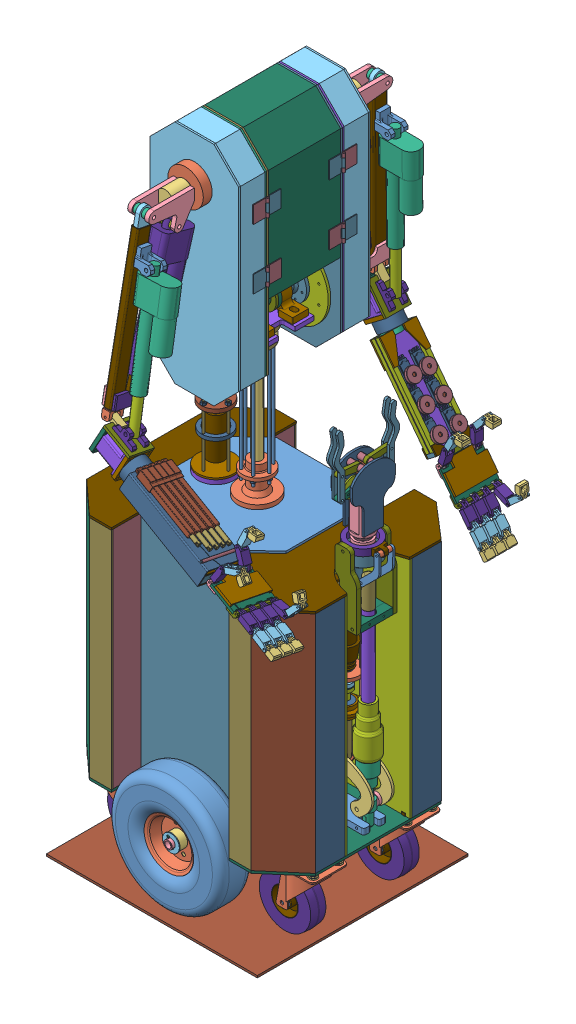
SolidWorks assembly sorbot, configuration По умолчанию. Lengths in mm. (continued)
Components (placement in the parent): (continued)
- bolt1-10: bolt1 [По умолчанию] at (-181.6432 28.2059 -219.1307) x (0.546944 0 -0.837169) z (-0.837169 0 -0.546944) size (14 40.5 16.17)
- bolt1-11: bolt1 [По умолчанию] at (-181.4767 28.2059 -278.9161) x (0.546944 0 -0.837169) z (-0.837169 0 -0.546944) size (14 40.5 16.17)
- bolt1-12: bolt1 [По умолчанию] at (-260.5141 28.2059 -278.9485) x (0.546944 0 -0.837169) z (-0.837169 0 -0.546944) size (14 40.5 16.17)
- bolt1-13: bolt1 [По умолчанию] at (-260.8842 28.1192 -54.1025) x (-0.546944 0 0.837169) z (0.837169 0 0.546944) size (14 40.5 16.17)
- bolt1-14: bolt1 [По умолчанию] at (-181.8952 28.1192 -54.0898) x (-0.546944 0 0.837169) z (0.837169 0 0.546944) size (14 40.5 16.17)
- bolt1-15: bolt1 [По умолчанию] at (-260.8825 28.1192 5.6198) x (-0.546944 0 0.837169) z (0.837169 0 0.546944) size (14 40.5 16.17)
- bolt1-16: bolt1 [По умолчанию] at (-181.994 28.1192 5.6123) x (-0.546944 0 0.837169) z (0.837169 0 0.546944) size (14 40.5 16.17)
- bolt1.nut-1: bolt1.nut [По умолчанию] at (-181.4767 51.9368 -278.9161) x (0 0 1) z (-1 0 0) size (14 6 16.17)
- bolt1.nut-2: bolt1.nut [По умолчанию] at (-260.5141 51.9368 -278.9485) x (0 0 1) z (-1 0 0) size (14 6 16.17)
- bolt1.nut-3: bolt1.nut [По умолчанию] at (-260.5376 51.9368 -219.1987) x (0 0 1) z (-1 0 0) size (14 6 16.17)
- bolt1.nut-4: bolt1.nut [По умолчанию] at (-181.6432 51.9368 -219.1307) x (0 0 1) z (-1 0 0) size (14 6 16.17)
- bolt1.nut-5: bolt1.nut [По умолчанию] at (-181.994 51.9368 5.6123) x (0 0 -1) z (1 0 0) size (14 6 16.17)
- bolt1.nut-6: bolt1.nut [По умолчанию] at (-260.8825 51.9368 5.6198) x (0 0 -1) z (1 0 0) size (14 6 16.17)
- bolt1.nut-7: bolt1.nut [По умолчанию] at (-260.8842 51.9368 -54.1025) x (0 0 -1) z (1 0 0) size (14 6 16.17)
- bolt1.nut-8: bolt1.nut [По умолчанию] at (-181.8952 51.9368 -54.0898) x (0 0 -1) z (1 0 0) size (14 6 16.17)
- bolt1.nut-9: bolt1.nut [По умолчанию] at (172.9115 51.9368 3.3236) x (0 0 -1) z (1 0 0) size (14 6 16.17)
- bolt1.nut-10: bolt1.nut [По умолчанию] at (251.9125 51.7388 3.3175) x (0 0 -1) z (1 0 0) size (14 6 16.17)
- bolt1.nut-11: bolt1.nut [По умолчанию] at (252.2608 51.5573 -56.3731) x (0 0 -1) z (1 0 0) size (14 6 16.17)
- bolt1.nut-12: bolt1.nut [По умолчанию] at (172.9018 51.3675 -56.2899) x (0 0 -1) z (1 0 0) size (14 6 16.17)
- bolt1.nut-13: bolt1.nut [По умолчанию] at (172.7558 51.9368 -277.7529) x (0 0 1) z (-1 0 0) size (14 6 16.17)
- bolt1.nut-14: bolt1.nut [По умолчанию] at (172.7717 51.9368 -218.0055) x (0 0 1) z (-1 0 0) size (14 6 16.17)
- bolt1.nut-15: bolt1.nut [По умолчанию] at (251.718 51.9368 -277.7613) x (0 0 1) z (-1 0 0) size (14 6 16.17)
- bolt1.nut-16: bolt1.nut [По умолчанию] at (251.8056 51.9368 -218.1439) x (0 0 1) z (-1 0 0) size (14 6 16.17)
- turret.table-1: turret.table [По умолчанию] at (-20.0648 607.7934 -136.9555) size (304.13 5 277.12)
- turret.center-1: turret.center [По умолчанию] at (-20.0648 607.7934 -136.9555) x (1 0 -0.000338) z (0.000338 0 1) size (90 80 90)
- body.center-1: body.center [По умолчанию] at (-20.0648 627.0246 -136.9555) size (22 355 22)
- wheel.axis.frame.fixture.p1-1: wheel.axis.frame.fixture.p1 [По умолчанию] at (40.6964 23.6368 -47.3934) x (0.999999 0 0.001149) z (-0.001149 0 0.999999) size (21.7 48.8 22.74)
- wheel.axis.frame.fixture.p1-2: wheel.axis.frame.fixture.p1 [По умолчанию] at (-54.5345 23.6368 -47.3503) size (21.7 48.8 22.74)
- wheel.axis.frame.fixture.p1-3: wheel.axis.frame.fixture.p1 [По умолчанию] at (40.6515 23.6368 -224.9519) size (21.7 48.8 22.74)
- wheel.axis.frame.fixture.p1-4: wheel.axis.frame.fixture.p1 [По умолчанию] at (-54.2945 23.6368 -224.8346) size (21.7 48.8 22.74)
- gearmotor.fixture.p2.1-1: gearmotor.fixture.p2.1 [По умолчанию] at (2.1309 53.4368 -208.1692) x (-1 0 0) z (0 0 -1) size (86 101.43 182)
- wheel.axis.frame.fixture.p2-1: wheel.axis.frame.fixture.p2 [По умолчанию] at (40.6964 51.9368 -47.3934) size (22.08 10 22.5)
- wheel.axis.frame.fixture.p2-2: wheel.axis.frame.fixture.p2 [По умолчанию] at (40.6515 53.4933 -224.9519) size (22.08 10 22.5)
- wheel.axis.frame.fixture.p2-3: wheel.axis.frame.fixture.p2 [По умолчанию] at (-54.2945 53.4933 -224.8346) size (22.08 10 22.5)
- wheel.axis.frame.fixture.p2-4: wheel.axis.frame.fixture.p2 [По умолчанию] at (-54.5345 53.4933 -47.3503) size (22.08 10 22.5)
- wall-fixture-3-2: wall-fixture-3 [По умолчанию] at (-150.6756 56.9368 4.4522) size (287.58 65 40)
- wall-fixture-3-1-1: wall-fixture-3-1 [По умолчанию] at (-154.6756 56.9368 4.4522) x (0 0 -1) z (1 0 0) size (74 65 40)
- wall-fixture-3-2-1: wall-fixture-3-2 [По умолчанию] at (-154.6756 56.9368 74.4522) size (42 65 40)
- wall-fixture-3-3-1: wall-fixture-3-3 [По умолчанию] at (-194.4824 56.9368 75.4251) x (0.73854 0 0.67421) z (-0.67421 0 0.73854) size (116.95 65 40)
- ground-1: ground [По умолчанию] at (-17.2598 -128.0632 -134.3184) size (500 5 500)
- body_pivot_fixture-1: body_pivot_fixture [По умолчанию] at (-20.0648 922.0246 -136.9555) x (0.99898 0 -0.04516) z (0.04516 0 0.99898) size (78 60 78)
- body_axis-1: body_axis [По умолчанию] at (-20.0648 1016.5246 -221.0975) x (0.999995 0.003042 0) z (0 0 1) size (21.8 21.8 170.35)
- body_tilt_drive_frame_p1-1: body_tilt_drive_frame_p1 [По умолчанию] at (-114.5063 612.7934 -276.3211) x (0.999999 0 0.001245) z (-0.001245 0 0.999999) size (186.87 100 2.5) (hidden)
- body_tilt_drive_frame_p1-2: body_tilt_drive_frame_p1 [По умолчанию] at (72.3667 612.7934 0.7968) x (-1 0 0) z (0 0 -1) size (186.87 100 2.5) (hidden)
- body_tilt_drive_frame_p2-1: body_tilt_drive_frame_p2 [По умолчанию] at (-169.9731 612.7934 -54.6628) x (0.72933 0 0.684163) z (-0.684163 0 0.72933) size (80.39 100 2.5) (hidden)
- body_tilt_drive_frame_p2-2: body_tilt_drive_frame_p2 [По умолчанию] at (-169.9731 712.7934 -220.8616) x (0.72933 0 -0.684163) z (-0.684163 0 -0.72933) size (80.39 100 2.5) (hidden)
- body_tilt_drive_frame_p3-1: body_tilt_drive_frame_p3 [По умолчанию] at (-173.1373 612.7934 -144.4799) x (0 0 -1) z (1 0 0) size (167.12 100 2.5) (hidden)
- body_tilt_drive_frame_p4-1: body_tilt_drive_frame_p4 [По умолчанию] at (130.9977 612.7934 -221.3211) x (0 0 1) z (-1 0 0) size (167.12 100 2.5) (hidden)
- body_tilt_drive_frame_p5-1: body_tilt_drive_frame_p5 [По умолчанию] at (65.0237 612.7934 -7.7276) x (0.72933 0 -0.684163) z (0.684163 0 0.72933) size (80.39 100 2.5) (hidden)
- body_tilt_drive_frame_p5-2: body_tilt_drive_frame_p5 [По умолчанию] at (78.6946 612.7934 -282.3701) x (0.72933 0 0.684163) z (-0.684163 0 0.72933) size (80.39 100 2.5) (hidden)
- turret.table.cap-1: turret.table.cap [По умолчанию] at (-20.0648 712.7934 -136.9555) size (304.13 2.5 277.12) (hidden)
- body_tilt_drive_frame_p6-2: body_tilt_drive_frame_p6 [По умолчанию] at (-175.1373 715.2934 -67.4448) x (1 0 0) z (0 0 1) size (300.14 367.75 2.5) (hidden)
- body_tilt_drive_frame_cap-1: body_tilt_drive_frame_cap [По умолчанию] at (-171.1373 715.2934 -64.9448) x (1 0 0) z (0 0 1) size (304.13 369.75 142) (hidden)
- body.frame.p1.fixture-1: body.frame.p1.fixture [По умолчанию] at (-20.8083 1016.2071 -56.7442) x (-0.989237 -0.146324 0) z (0 0 -1) size (89 89 22)
- body.frame.p1.fixture-2: body.frame.p1.fixture [По умолчанию] at (-20.0648 1016.5246 -216.3595) x (0.862438 0.506162 0) z (0 0 1) size (89 89 22)
- body.frame.p2-1: body.frame.p2 [По умолчанию] at (-4.2156 797.7971 -50.7442) x (-1 0 0) z (0 0 -1) size (210 323.57 171.62)
- body.frame.p3-1: body.frame.p3 [По умолчанию] at (94.3623 1112.7235 -40.8506) x (-1 0 0) z (0 0 -1) size (206 2 171.62)
- arm.actuator-1: arm.actuator [Default] at (-99.8542 1094.2549 -11.7544) x (0 0 -1) z (0.997731 -0.067324 0) size (42 292 82)
  - arm.actuator.p1-1: arm.actuator.p1 [Default] at (1.9897 -28.1276 18.0595) size (42 292 82)
- arm.actuator.p2-1: arm.actuator.p2 [Default] at (-71.2141 1250.4494 -13.7442) x (-0.997731 0.067324 0) z (0 0 -1) size (20 180 20)
- arm.lift.actuator.fixture.p2-1: arm.lift.actuator.fixture.p2 [По умолчанию] at (-88.5767 993.1387 -41.8307) x (0.99962 0.027553 0) z (0 0 1) size (8 8 57)
- shoulder.p4-1: shoulder.p4 [По умолчанию] at (-12.6529 1335.4871 -25.7442) x (0.590367 -0.807135 0) z (0 0 1) size (124.11 60 4)
- shoulder.p4-2: shoulder.p4 [По умолчанию] at (-12.6483 1335.4904 -1.7442) x (0.590423 -0.807094 0) z (0 0 1) size (124.11 60 4)
- arm.lift.actuator.fixture.p3-1: arm.lift.actuator.fixture.p3 [По умолчанию] at (-88.5767 993.1387 15.2558) x (-1 -0.000227 0) z (0 0 -1) size (39.1 39.1 19)
- arm.lift.actuator.fixture.p3-2: arm.lift.actuator.fixture.p3 [По умолчанию] at (-88.5767 993.1387 -42.7442) x (1 -0.000113 0) z (0 0 1) size (39.1 39.1 19)
- shoulder.p6-1: shoulder.p6 [По умолчанию] at (-12.6457 1335.4135 -42.7442) x (-0.13701 -0.99057 0) z (0 0 1) size (53.6 53.6 22)
- shoulder.p6-2: shoulder.p6 [По умолчанию] at (-12.6483 1335.4904 16.6679) x (-0.526603 0.850111 0) z (0 0 -1) size (53.6 53.6 22)
- body.frame.p5-1: body.frame.p5 [По умолчанию] at (-12.763 795.3888 -42.7442) x (1 0 0) z (0 0 1) size (210 537.69 58)
- arm.actuator-2: arm.actuator [Default] at (-14.7745 1195.5912 125.5833) x (1 0 0) z (0 -0.279359 -0.960187) size (42 292 82)
  - arm.actuator.p1-1: arm.actuator.p1 [Default] at (1.9897 -28.1276 18.0595) size (42 292 82)
- arm.actuator.p2-2: arm.actuator.p2 [Default] at (-12.7848 1120.5046 128.6209) x (0 -0.279359 -0.960187) z (-1 0 0) size (20 180 20)
- arm.actuator100mm..p1-1: arm.actuator100mm..p1 [Default] at (32.1534 1179.3256 170.6338) x (0 0.190943 0.981601) z (0.999474 0.031845 -0.006195) size (42 244 82)
- arm.actuator100mm.p2-1: arm.actuator100mm.p2 [Default] at (35.8637 1067.1234 192.4596) x (0.999474 0.031845 -0.006195) z (0 -0.190943 -0.981601) size (20 130 20)
- forearm.rotate-1: forearm.rotate [Default] at (-12.4635 914.4269 195.3279) x (0.410922 0.894897 -0.174077) z (0 -0.190943 -0.981601) size (61.21 87 60)
  - SY57STH56-2804A-1: SY57STH56-2804A [Default] at (-3.5843 6.169 -26.3301) size (56 76.6 56)
  - forearm.rotate.p1-1: forearm.rotate.p1 [Default] at (-15.5843 62.169 -26.3301) size (61.21 8 60)
  - forearm.rotate.p4-1: forearm.rotate.p4 [Default] at (-3.5843 70.169 -26.3301) size (58 23 58)
- forearm.rotate.p2-1: forearm.rotate.p2 [Default] at (43.2427 890.9484 226.7186) x (-0.401682 -0.915039 -0.036821) z (-0.086648 -0.002051 0.996237) size (41 32 41)
- body.frame.p1-3: body.frame.p1 [По умолчанию] at (-12.5732 795.4676 -50.7442) x (1 0 0) z (0 0 1) size (210 537.56 4)
- cap-hinge-1: cap-hinge [По умолчанию] at (95.4017 1285.4557 -46.5922) x (0 0 1) z (0 1 0) size (35.83 6 40)
- cap-hinge-p1-1: cap-hinge-p1 [По умолчанию] at (95.4017 1326.2182 -46.5922) x (0 0 -1) z (0 -1 0) size (35.83 6 40)
- cap-hinge-2: cap-hinge [По умолчанию] at (95.4017 1183.4534 -46.8053) x (0 0 -1) z (0 -1 0) size (35.83 6 40)
- cap-hinge-p1-2: cap-hinge-p1 [По умолчанию] at (95.4017 1142.6154 -46.8053) x (0 0 1) z (0 1 0) size (35.83 6 40)
- forearm.rotate.p1.m1-1: forearm.rotate.p1.m1 [Default] at (-13.2433 903.0197 224.3704) x (0.410922 0.894897 -0.174077) z (0 0.190943 0.981601) size (61.21 8 60)
- forearm.rotate.p7-1: forearm.rotate.p7 [По умолчанию] at (-4.8958 950.8147 245.6356) x (0.410922 0.894897 -0.174077) z (0 0.190943 0.981601) size (6 72 60)
- forearm.rotate.p8-1: forearm.rotate.p8 [По умолчанию] at (-3.4001 950.887 215.0701) x (0.410922 0.894897 -0.174077) z (0 0.190943 0.981601) size (22.83 55.54 10)
- forearm.rotate.p8-2: forearm.rotate.p8 [По умолчанию] at (-3.4001 945.1587 185.622) x (0.410922 0.894897 -0.174077) z (0 0.190943 0.981601) size (22.83 55.54 10)
- arm.p1.m-1: arm.p1.m [По умолчанию] at (-12.763 1310.2593 145.0478) x (1 0 0) z (0 -0.190943 -0.981601) size (18 345 32.5)
- actuator.100.fixture-1: actuator.100.fixture [По умолчанию] at (23.3566 1239.3204 158.8469) x (0 0.190943 0.981601) z (-1 0 0) size (40 40 44)
- forearm.rotate.p9-1: forearm.rotate.p9 [По умолчанию] at (-4.2763 976.3165 172.7436) x (-1 0 0) z (0 0.190943 0.981601) size (18 53 34)
- forearm.rotate.p10-1: forearm.rotate.p10 [По умолчанию] at (-19.0339 954.2606 224.2315) x (0 -0.190943 -0.981601) z (0.911671 -0.403361 0.078463) size (18 10 35)
- forearm.rotate.p12-1: forearm.rotate.p12 [По умолчанию] at (-21.7679 955.7142 133.8743) x (1 0 0) z (0 -0.190943 -0.981601) size (7 35 61.58)
- forearm.rotate.p3-1: forearm.rotate.p3 [Default] at (64.9076 884.5938 209.967) x (-0.42896 0.179577 0.885294) z (0.863514 0.369251 0.343507) size (6 6 6)
- lower.arm.p1-1: lower.arm.p1 [По умолчанию] at (72.4162 878.0408 229.2294) x (0.911671 -0.403361 0.078463) z (0 0.190943 0.981601) size (10 32 66)
- lower.arm.p2-1: lower.arm.p2 [По умолчанию] at (74.8904 890.6651 265.5015) x (0.91167 -0.4031 0.079805) z (-0.001246 0.191494 0.981493) size (215 10 10)
- lower.arm.p2-2: lower.arm.p2 [По умолчанию] at (69.9594 879.9264 267.5905) x (0.91167 -0.4031 0.079805) z (-0.001246 0.191494 0.981493) size (215 10 10)
- lower.arm.p2-3: lower.arm.p2 [По умолчанию] at (74.873 876.1612 190.8982) x (0.91167 -0.4031 0.079805) z (-0.001246 0.191494 0.981493) size (215 10 10)
- lower.arm.p2-4: lower.arm.p2 [По умолчанию] at (69.9419 865.4224 192.9872) x (0.91167 -0.4031 0.079805) z (-0.001246 0.191494 0.981493) size (215 10 10)
- lower.arm.p3-1: lower.arm.p3 [По умолчанию] at (72.2851 869.3845 190.1638) x (0.91167 -0.4031 0.079805) z (-0.001246 0.191494 0.981493) size (215 2 86)
- lower.arm.p4-3: lower.arm.p4 [По умолчанию] at (66.2548 872.8298 274.0646) x (0.91167 -0.4031 0.079805) z (-0.001246 0.191494 0.981493) size (57.43 4 30.19)
- HS-311 Hitec Standard Servo and Horn-1: HS-311 Hitec Standard Servo and Horn [Default] at (137.9404 826.1872 257.502) x (-0.001246 0.191494 0.981493) z (-0.91167 0.4031 -0.079805) size (27.94 44.98 53.29)
  - HS-311 Hitec Standard Servo-1: HS-311 Hitec Standard Servo [Default] at origin size (20.32 41.27 53.29)
  - HS-311-p2-1: HS-311-p2 [По умолчанию] at (0 42.485 0) x (0.967717 0 0.252038) z (-0.252038 0 0.967717) size (22.63 6.25 24)
- HS-311 Hitec Standard Servo and Horn-2: HS-311 Hitec Standard Servo and Horn [Default] at (188.1296 796.7399 224.5945) x (-0.001246 0.191494 0.981493) z (-0.91167 0.4031 -0.079805) size (27.94 44.98 53.29)
  - HS-311 Hitec Standard Servo-1: HS-311 Hitec Standard Servo [Default] at origin size (20.32 41.27 53.29)
  - HS-311-p2-1: HS-311-p2 [По умолчанию] at (0 42.485 0) x (0.967717 0 0.252038) z (-0.252038 0 0.967717) size (22.63 6.25 24)
- HS-311 Hitec Standard Servo and Horn-3: HS-311 Hitec Standard Servo and Horn [Default] at (137.9846 819.3891 222.659) x (-0.001246 0.191494 0.981493) z (-0.91167 0.4031 -0.079805) size (27.94 44.98 53.29)
  - HS-311 Hitec Standard Servo-1: HS-311 Hitec Standard Servo [Default] at origin size (20.32 41.27 53.29)
  - HS-311-p2-1: HS-311-p2 [По умолчанию] at (0 42.485 0) x (0.967717 0 0.252038) z (-0.252038 0 0.967717) size (22.63 6.25 24)
- HS-311 Hitec Standard Servo and Horn-4: HS-311 Hitec Standard Servo and Horn [Default] at (238.2746 774.0787 226.4684) x (-0.001246 0.191494 0.981493) z (-0.91167 0.4031 -0.079805) size (27.94 44.98 53.29)
  - HS-311 Hitec Standard Servo-1: HS-311 Hitec Standard Servo [Default] at origin size (20.32 41.27 53.29)
  - HS-311-p2-1: HS-311-p2 [По умолчанию] at (0 42.485 0) x (0.967717 0 0.252038) z (-0.252038 0 0.967717) size (22.63 6.25 24)
- HS-311 Hitec Standard Servo and Horn-5: HS-311 Hitec Standard Servo and Horn [Default] at (188.0785 804.5912 264.8357) x (-0.001246 0.191494 0.981493) z (-0.91167 0.4031 -0.079805) size (27.94 44.98 53.29)
  - HS-311 Hitec Standard Servo-1: HS-311 Hitec Standard Servo [Default] at origin size (20.32 41.27 53.29)
  - HS-311-p2-1: HS-311-p2 [По умолчанию] at (0 42.485 0) x (0.967717 0 0.252038) z (-0.252038 0 0.967717) size (22.63 6.25 24)
- HS-311 Hitec Standard Servo and Horn-6: HS-311 Hitec Standard Servo and Horn [Default] at (238.2177 782.8261 271.303) x (-0.001246 0.191494 0.981493) z (-0.91167 0.4031 -0.079805) size (27.94 44.98 53.29)
  - HS-311 Hitec Standard Servo-1: HS-311 Hitec Standard Servo [Default] at origin size (20.32 41.27 53.29)
  - HS-311-p2-1: HS-311-p2 [По умолчанию] at (0 42.485 0) x (0.967717 0 0.252038) z (-0.252038 0 0.967717) size (22.63 6.25 24)
- forearm.rotate.p17-2: forearm.rotate.p17 [По умолчанию] at (88.654 871.0225 197.0126) x (0.91167 -0.4031 0.079805) z (-0.001246 0.191494 0.981493) size (10 10 66)
- forearm.rotate.p17-3: forearm.rotate.p17 [По умолчанию] at (83.7229 860.2838 199.1015) x (0.91167 -0.4031 0.079805) z (-0.001246 0.191494 0.981493) size (10 10 66)
- lower.arm.p4-5: lower.arm.p4 [По умолчанию] at (76.9388 896.0971 269.5386) x (0.91167 -0.4031 0.079805) z (-0.001246 0.191494 0.981493) size (57.43 4 30.19)
- lower.arm.p4-6: lower.arm.p4 [По умолчанию] at (78.5775 883.2578 184.4241) x (0.91167 -0.4031 0.079805) z (0.001246 -0.191494 -0.981493) size (57.43 4 30.19)
- lower.arm.p4-7: lower.arm.p4 [По умолчанию] at (67.8935 859.9904 188.9501) x (0.91167 -0.4031 0.079805) z (0.001246 -0.191494 -0.981493) size (57.43 4 30.19)
- lower.arm.p9-1: lower.arm.p9 [По умолчанию] at (154.3711 861.9696 250.5415) x (0.91167 -0.4031 0.079805) z (-0.001246 0.191494 0.981493) size (32.15 8 32.15)
- lower.arm.p9-2: lower.arm.p9 [По умолчанию] at (154.4153 855.1716 215.6985) x (0.91167 -0.4031 0.079805) z (-0.001246 0.191494 0.981493) size (32.15 8 32.15)
- lower.arm.p9-3: lower.arm.p9 [По умолчанию] at (254.6484 818.6086 264.3425) x (0.91167 -0.4031 0.079805) z (-0.001246 0.191494 0.981493) size (32.15 8 32.15)
- lower.arm.p9-4: lower.arm.p9 [По умолчанию] at (204.5092 840.3736 257.8752) x (0.91167 -0.4031 0.079805) z (-0.001246 0.191494 0.981493) size (32.15 8 32.15)
- lower.arm.p9-5: lower.arm.p9 [По умолчанию] at (204.5603 832.5224 217.634) x (0.91167 -0.4031 0.079805) z (-0.001246 0.191494 0.981493) size (32.15 8 32.15)
- lower.arm.p9-6: lower.arm.p9 [По умолчанию] at (254.7053 809.8611 219.5079) x (0.91167 -0.4031 0.079805) z (-0.001246 0.191494 0.981493) size (32.15 8 32.15)
- lower.arm.p8-2: lower.arm.p8 [По умолчанию] at (272.9478 809.4306 286.6966) x (0.91167 -0.4031 0.079805) z (-0.001246 0.191494 0.981493) size (8 36.31 86)
- palm.p1-3: palm.p1 [По умолчанию] at (322.748 783.4115 260.2518) x (0.91167 -0.4031 0.079805) z (-0.001246 0.191494 0.981493) size (75 6 100)
- palm.p3-1: palm.p3 [По умолчанию] at (365.8383 752.7967 227.563) x (-0.001246 0.191494 0.981493) z (-0.91167 0.4031 -0.079805) size (100 13.5 26)
- finger.p1-1: finger.p1 [По умолчанию] at (361.4047 778.3293 288.0374) x (0.91167 -0.4031 0.079805) z (-0.001246 0.191494 0.981493) size (50 12 20.5)
- palm.fixture.p4-1: palm.fixture.p4 [По умолчанию] at (280.2412 806.2058 287.335) x (0.001246 -0.191494 -0.981493) z (0.91167 -0.4031 0.079805) size (25 4 20)
- palm.fixture.p4-3: palm.fixture.p4 [По умолчанию] at (269.5572 782.9385 291.861) x (0.001246 -0.191494 -0.981493) z (0.91167 -0.4031 0.079805) size (25 4 20)
- palm.fixture.p4-4: palm.fixture.p4 [По умолчанию] at (280.3484 789.7373 202.9266) x (-0.91167 0.4031 -0.079805) z (0.001246 -0.191494 -0.981493) size (25 4 20)
- palm.fixture.p4-5: palm.fixture.p4 [По умолчанию] at (271.1797 769.7699 206.8107) x (-0.001246 0.191494 0.981493) z (0.91167 -0.4031 0.079805) size (25 4 20)
- finger.spring-1: finger.spring [По умолчанию] at (365.5538 775.1528 287.2462) x (-0.410922 -0.894897 0.174077) z (-0.001246 0.191494 0.981493) size (5.38 21 4.23)
- palm.fixture.p13-1: palm.fixture.p13 [По умолчанию] at (365.5375 777.6582 300.0875) x (-0.290544 -0.939223 0.182878) z (0.001246 -0.191494 -0.981493) size (3 3 100)
- finger.spring-2: finger.spring [По умолчанию] at (401.7674 756.3188 288.6743) x (-0.396016 -0.901345 0.175354) z (-0.001246 0.191494 0.981493) size (5.38 21 4.23)
- finger.p3-1: finger.p3 [По умолчанию] at (433.9086 745.1991 294.7083) x (0.91167 -0.403099 0.079804) z (-0.001246 0.191494 0.981493) size (30 12 20.5)
- finger.p1-2: finger.p1 [По умолчанию] at (360.8897 762.5687 213.1692) x (0.98549 -0.16635 0.033707) z (-0.001246 0.191494 0.981493) size (50 12 20.5)
- finger.p3-2: finger.p3 [По умолчанию] at (431.7485 777.5134 210.4584) x (-0.381637 0.907115 -0.177467) z (-0.001246 0.191494 0.981493) size (30 12 20.5)
- finger.p1-3: finger.p1 [По умолчанию] at (361.4364 773.4462 263.0093) x (0.91167 -0.4031 0.079805) z (-0.001246 0.191494 0.981493) size (50 12 20.5)
- finger.p3-3: finger.p3 [По умолчанию] at (434.2984 741.0676 269.547) x (0.91167 -0.403099 0.079804) z (-0.001246 0.191494 0.981493) size (30 12 20.5)
- palm.p3.m-1: palm.p3.m [По умолчанию] at (290.0454 800.8206 295.5301) x (0.001246 -0.191494 -0.981493) z (0.91167 -0.4031 0.079805) size (21.5 12 26)
- finger.p1-4: finger.p1 [По умолчанию] at (361.4682 768.5631 237.9812) x (0.91167 -0.4031 0.079805) z (-0.001246 0.191494 0.981493) size (50 12 20.5)
- finger.p3-4: finger.p3 [По умолчанию] at (434.4109 736.3198 244.285) x (0.91167 -0.403099 0.079804) z (-0.001246 0.191494 0.981493) size (30 12 20.5)
- palm.p3.m-2: palm.p3.m [По умолчанию] at (290.1432 785.7883 218.4829) x (0.001246 -0.191494 -0.981493) z (0.91167 -0.4031 0.079805) size (21.5 12 26)
- finger.p1-5: finger.p1 [По умолчанию] at (295.6891 799.1773 284.9052) x (0.507409 0.845879 -0.164391) z (0.001246 -0.191494 -0.981493) size (50 12 20.5)
- finger.p3-5: finger.p3 [По умолчанию] at (350.9841 851.791 274.8252) x (0.60933 -0.778097 0.152584) z (0.001246 -0.191494 -0.981493) size (30 12 20.5)
- finger.p1-6: finger.p1 [По умолчанию] at (300.6579 784.9923 207.8008) x (-0.461749 0.870485 -0.170422) z (0.001246 -0.191494 -0.981493) size (50 12 20.5)
- finger.p3-6: finger.p3 [По умолчанию] at (287.4487 858.7406 193.5103) x (0.994901 -0.09875 0.02053) z (0.001246 -0.191494 -0.981493) size (30 12 20.5)
- finger.p2-7: finger.p2 [По умолчанию] at (398.8681 761.8903 291.2923) x (0.900656 -0.426275 0.084312) z (-0.001246 0.191494 0.981493) size (48 12 20.5)
- finger.p2-8: finger.p2 [По умолчанию] at (398.8292 756.9343 266.2783) x (0.909838 -0.407065 0.080576) z (-0.001246 0.191494 0.981493) size (48 12 20.5)
- finger.p2-9: finger.p2 [По умолчанию] at (398.8449 752.0341 241.2536) x (0.911901 -0.402596 0.079707) z (-0.001246 0.191494 0.981493) size (48 12 20.5)
- finger.p2-10: finger.p2 [По умолчанию] at (401.3615 751.2293 215.433) x (0.665201 0.733005 -0.142168) z (-0.001246 0.191494 0.981493) size (48 12 20.5)
- finger.p2-11: finger.p2 [По умолчанию] at (313.5856 835.7577 277.7909) x (0.959794 0.275737 -0.052579) z (0.001246 -0.191494 -0.981493) size (48 12 20.5)
- finger.p2-12: finger.p2 [По умолчанию] at (278.1338 819.2671 201.085) x (0.352805 0.918465 -0.178749) z (0.001246 -0.191494 -0.981493) size (48 12 20.5)
- finger1.rod-1: finger1.rod [По умолчанию] at (451.9435 740.6273 293.9037) x (0.91167 -0.403099 0.079804) z (-0.001246 0.191494 0.981493) size (196.04 3.19 32.22)
- palm.p5-1: palm.p5 [По умолчанию] at (331.4609 789.3117 276.6833) x (0.91167 -0.4031 0.079805) z (-0.001246 0.191494 0.981493) size (21.8 4 21.8)
- palm.p6-1: palm.p6 [По умолчанию] at (302.9044 799.3879 261.0737) x (0.91167 -0.4031 0.079805) z (-0.001246 0.191494 0.981493) size (13.8 4 13.8)
- palm.p5-2: palm.p5 [По умолчанию] at (331.5169 778.2186 219.7881) x (0.91167 -0.4031 0.079805) z (-0.001246 0.191494 0.981493) size (21.8 4 21.8)
- palm.p6-2: palm.p6 [По умолчанию] at (302.8729 793.2734 229.5656) x (0.91167 -0.4031 0.079805) z (-0.001246 0.191494 0.981493) size (13.8 4 13.8)
- palm.cap-1: palm.cap [По умолчанию] at (361.633 779.9337 299.6962) x (0.91167 -0.4031 0.079805) z (-0.001246 0.191494 0.981493) size (62.89 6 100)
- arm.cap-1: arm.cap [По умолчанию] at (82.2621 895.7683 208.6072) x (0.91167 -0.4031 0.079805) z (-0.001246 0.191494 0.981493) size (223 41 91)
- finger.actuator.p1-3: finger.actuator.p1 [По умолчанию] at (95.0081 909.8486 253.6334) x (0.001246 -0.191494 -0.981493) z (0.91167 -0.4031 0.079805) size (15 18 153)
- finger.actuator.p2-5: finger.actuator.p2 [По умолчанию] at (149.1541 885.9077 258.3732) x (-0.001246 0.191494 0.981493) z (0.410922 0.894897 -0.174077) size (9 107.09 9)
- finger.actuator.p1-4: finger.actuator.p1 [По умолчанию] at (95.0455 904.1038 224.1887) x (0.001246 -0.191494 -0.981493) z (0.91167 -0.4031 0.079805) size (15 18 153)
- finger.actuator.p2-6: finger.actuator.p2 [По умолчанию] at (164.0617 873.5879 230.2301) x (-0.001246 0.191494 0.981493) z (0.410922 0.894897 -0.174077) size (9 107.09 9)
- finger.actuator.p1-5: finger.actuator.p1 [По умолчанию] at (95.0268 906.9762 238.911) x (0.001246 -0.191494 -0.981493) z (0.91167 -0.4031 0.079805) size (15 18 153)
- finger.actuator.p2-7: finger.actuator.p2 [По умолчанию] at (162.8681 876.9798 244.8496) x (-0.001246 0.191494 0.981493) z (0.410922 0.894897 -0.174077) size (9 107.09 9)
- finger.actuator.p1-6: finger.actuator.p1 [По умолчанию] at (95.0829 898.3589 194.7439) x (0.001246 -0.191494 -0.981493) z (0.91167 -0.4031 0.079805) size (15 18 153)
- finger.actuator.p2-8: finger.actuator.p2 [По умолчанию] at (164.758 867.5517 200.843) x (-0.001246 0.191494 0.981493) z (0.410922 0.894897 -0.174077) size (9 107.09 9)
- finger.actuator.p1-7: finger.actuator.p1 [По умолчанию] at (95.0642 901.2314 209.4663) x (0.001246 -0.191494 -0.981493) z (0.91167 -0.4031 0.079805) size (15 18 153)
- finger.actuator.p2-9: finger.actuator.p2 [По умолчанию] at (164.458 870.5485 215.5408) x (-0.001246 0.191494 0.981493) z (0.410922 0.894897 -0.174077) size (9 107.09 9)
- fingers.fixture.p2-2: fingers.fixture.p2 [По умолчанию] at (272.124 815.755 202.6327) x (0.877417 0.471059 -0.090792) z (-0.001246 0.191494 0.981493) size (6 6 86)
- fingers.fixture.p1-2: fingers.fixture.p1 [По умолчанию] at (272.1386 813.5138 191.1453) x (0.91167 -0.403099 0.079804) z (-0.001246 0.191494 0.981493) size (3.5 3.5 100)
- finger.rod.2-1: finger.rod.2 [По умолчанию] at (241.0115 844.8178 266.5403) x (0.91167 -0.403099 0.079804) z (-0.001246 0.191494 0.981493) size (153.47 13.84 32.76)
- palm.fixture.p14-1: palm.fixture.p14 [По умолчанию] at (281.009 802.4403 259.5427) x (0.91167 -0.4031 0.079805) z (-0.001246 0.191494 0.981493) size (37 23.78 30)
- forearm.rotate.p12-m-1: forearm.rotate.p12-m [По умолчанию] at (3.237 955.7142 133.8743) x (1 0 0) z (0 -0.190943 -0.981601) size (7 30.01 61.58)
- arm.fixture.cap-1: arm.fixture.cap [По умолчанию] at (-12.4559 1335.4922 -51.2442) x (0.999995 -0.003183 0) z (0.003183 0.999995 0) size (110 23 110)
- body_tilit_stud-1: body_tilit_stud [По умолчанию] at (-48.2188 648.7352 -136.446) x (1 0 -0.000338) z (0.000338 0 1) size (6 307 6)
- body_tilt_drive_frame_p6-3: body_tilt_drive_frame_p6 [По умолчанию] at (-175.1373 715.2934 -206.9448) x (1 0 0) z (0 0 1) size (300.14 367.75 2.5) (hidden)
- shoulder.bearing.housing-1: shoulder.bearing.housing [По умолчанию] at (-12.7629 1335.3853 19.2558) x (1 0 0) z (0 0 1) size (84 84 21)
- shoulder.bearing.housing-2: shoulder.bearing.housing [По умолчанию] at (-12.4903 1335.516 -46.7442) x (-0.799769 0.600308 0) z (0 0 -1) size (84 84 21)
- shoulder.axis-1: shoulder.axis [По умолчанию] at (-12.7629 1335.3853 -67.7442) x (1 0 0) z (0 0 1) size (30 40 157)
- arm.fixture-2: arm.fixture [По умолчанию] at (-27.7629 1348.6141 44.2558) x (-1 0 0) z (0 0 -1) size (10 73.07 108.23)
- shoulder.lever-1: shoulder.lever [По умолчанию] at (-7.763 1343.4657 102.1683) x (-1 0 0) z (0 -0.190943 -0.981601) size (10 77.8 28.5)
- arm.lift2.actuator.fixture.p1-1: arm.lift2.actuator.fixture.p1 [По умолчанию] at (-27.763 1335.3853 140.1602) x (1 0 0) z (0 -0.000978 1) size (10 20 20)
- arm.lift2.actuator.fixture.p1.m1-1: arm.lift2.actuator.fixture.p1.m1 [По умолчанию] at (-27.7629 1286.6873 80.2712) x (1 0 0) z (0 -0.000962 1) size (5 20 20)
- arm.fixture-3: arm.fixture [По умолчанию] at (12.2371 1348.614 44.2558) x (-1 0 0) z (0 0 -1) size (10 73.07 108.23)
- arm.lift2.actuator.fixture.p1-3: arm.lift2.actuator.fixture.p1 [По умолчанию] at (-7.7629 1335.3853 140.1602) x (1 0 0) z (0 -0.000978 1) size (10 20 20)
- arm.lift2.actuator.fixture.p1.m1-2: arm.lift2.actuator.fixture.p1.m1 [По умолчанию] at (-2.7629 1286.6873 80.2712) x (1 0 0) z (0 -0.000962 1) size (5 20 20)
- body_pivot-2: body_pivot [По умолчанию] at (-55.8885 972.0246 -153.8981) x (1 0 0) z (0 0 1) size (140 10 130)
- body.tilt.axis.frame-2: body.tilt.axis.frame [По умолчанию] at (29.9352 1018.0246 -79.5942) x (-1 0 0) z (0 0 -1) size (126 65.5 38)
- body.tilt.axis.frame-3: body.tilt.axis.frame [По умолчанию] at (-70.0648 1018.0246 -194.4875) x (1 0 0) z (0 0 1) size (126 65.5 38)
- tilt.thread.rod-1: tilt.thread.rod [По умолчанию] at (-118.5699 729.5591 -137.5376) x (0.714335 0 -0.699804) z (0.699804 0 0.714335) size (18.48 155.29 16)
- tilt.thread.rod.fixture.2-1: tilt.thread.rod.fixture.2 [По умолчанию] at (-118.5699 793.5591 -137.5376) size (40 26 40)
- tilit.thread.rod.bearing.fixture-1: tilit.thread.rod.bearing.fixture [По умолчанию] at (-130.6447 929.0246 -154.0466) x (0.999985 0 0.005494) z (-0.005494 0 0.999985) size (171.17 8 70)
- tilit.thread.bearing-1: tilit.thread.bearing [По умолчанию] at (-118.5699 937.0246 -137.5376) size (28 8 28)
- tilit.thread.rod.bearing.housing-1: tilit.thread.rod.bearing.housing [По умолчанию] at (-118.5699 937.0246 -137.5376) size (42.5 10 42.5)
- body_tilt_axis_clamp-1: body_tilt_axis_clamp [По умолчанию] at (-20.0648 1016.5246 -90.4875) x (-0.92275 -0.3854 0) z (0 0 -1) size (65 65 23)
- body_tilt_axis_clamp-2: body_tilt_axis_clamp [По умолчанию] at (-20.0648 1016.5246 -183.5942) x (0.999995 0.003042 0) z (0 0 1) size (65 65 23)
- body_tilt_lever-1: body_tilt_lever [По умолчанию] at (-20.0648 1016.5246 -155.4875) x (0.894303 0.447461 0) z (0 0 1) size (137.08 65 6)
- body_tilt_lever-2: body_tilt_lever [По умолчанию] at (-20.0648 1016.5246 -124.5942) x (0.894303 0.447461 0) z (0 0 1) size (137.08 65 6)
- body.tilit.lever.2-1: body.tilit.lever.2 [По умолчанию] at (-118.5699 828.2928 -177.3819) x (0.12832 0.991733 0) z (-0.991733 0.12832 0) size (179.8 7 30)
- body_tilt_lever_axis-1: body_tilt_lever_axis [По умолчанию] at (-99.3474 976.856 -195.4875) x (-0.131453 -0.991322 0) z (0 0 1) size (10 10 115)
- body.tilt.nut-1: body.tilt.nut [По умолчанию] at (-118.5699 828.2928 -137.5376) x (1 0 -0.000625) z (0.000625 0 1) size (36 14 31.19)
- body.tilit.nut.housing-1: body.tilit.nut.housing [По умолчанию] at (-118.5699 818.2928 -137.5376) x (0 0 -1) z (1 0 0) size (79.69 20 43.97)
- body.tilit.nut.housing.bolt-1: body.tilit.nut.housing.bolt [По умолчанию] at (-118.5699 828.2928 -184.3819) x (0 0 1) z (-1 0 0) size (38 19.4 20.53)
- body.tilit.nut.housing.cap-1: body.tilit.nut.housing.cap [По умолчанию] at (-96.5829 838.2928 -177.3819) x (0 0 1) z (-1 0 0) size (79.69 10 43.97)
- body.tilit.extender-1: body.tilit.extender [По умолчанию] at (-99.3474 976.856 -155.4875) x (0 0 -1) z (1 0 0) size (21.5 30 30)
- washer-1: washer [По умолчанию] at (-99.3474 976.856 -186.3819) x (1 0 0) z (0 0 1) size (24 24 2)
- body.tilit.extender-2: body.tilit.extender [По умолчанию] at (-99.3474 976.856 -97.0942) x (0 0 -1) z (1 0 0) size (21.5 30 30)
- body.tilit.lever.2-2: body.tilit.lever.2 [По умолчанию] at (-118.5699 828.2928 -90.6932) x (0.12832 0.991733 0) z (-0.991733 0.12832 0) size (179.8 7 30)
- body.tilit.nut.housing.bolt-2: body.tilit.nut.housing.bolt [По умолчанию] at (-118.5699 828.2928 -90.6932) x (0 0 -1) z (1 0 0) size (38 19.4 20.53)
- washer-2: washer [По умолчанию] at (-99.3474 976.856 -90.6932) x (1 0 0) z (0 0 1) size (24 24 2)
- body.tilit.enforcement-1: body.tilit.enforcement [По умолчанию] at (-20.8083 1016.2071 -56.7442) x (0.999986 -0.005204 0) z (-0.005204 -0.999986 0) size (178 6 178)
- body.tilit.enforcement-2: body.tilit.enforcement [По умолчанию] at (-20.0648 1016.5246 -222.3595) x (1 0 0) z (0 -1 0) size (178 6 178)
- arm.fixture.cap-2: arm.fixture.cap [По умолчанию] at (-15.2428 1335.4923 -221.8595) x (0.999986 -0.005204 0) z (-0.005204 -0.999986 0) size (110 23 110)
- body.frame.p4-4: body.frame.p4 [По умолчанию] at (-12.3773 795.5195 -230.3595) x (1 0 0) z (0 0 1) size (210 537.56 4)
- body.frame.p5-2: body.frame.p5 [По умолчанию] at (-12.6499 795.3889 -288.3595) x (1 0 0) z (0 0 1) size (210 537.69 58)
- cap-hinge-p1-3: cap-hinge-p1 [По умолчанию] at (95.5097 1287.1115 -226.3787) x (0 0 1) z (0 1 0) size (35.83 6 40)
- cap-hinge-4: cap-hinge [По умолчанию] at (95.5097 1143.1735 -226.3787) x (0 0 1) z (0 1 0) size (35.83 6 40)
- cap-hinge-5: cap-hinge [По умолчанию] at (95.5097 1327.9494 -226.3787) x (-0.005204 0 -0.999986) z (0 -1 0) size (35.83 6 40)
- cap-hinge-p1-4: cap-hinge-p1 [По умолчанию] at (95.5097 1183.936 -226.3787) x (-0.005211 0 -0.999986) z (0 -1 0) size (35.83 6 40)
- shoulder.bearing.housing-3: shoulder.bearing.housing [По умолчанию] at (-12.6499 1335.3853 -292.3595) x (1 -0.000001 0) z (0 0 -1) size (84 84 21)
- shoulder.bearing.housing-4: shoulder.bearing.housing [По умолчанию] at (-12.3772 1335.516 -226.3595) x (1 0 0) z (0 0 1) size (84 84 21)
- shoulder.axis-2: shoulder.axis [По умолчанию] at (-12.6499 1335.3853 -205.3595) x (1 0 0) z (0 0 -1) size (30 40 157)
- shoulder.p6-3: shoulder.p6 [По умолчанию] at (-12.6499 1335.3853 -227.2739) x (-0.950595 -0.310432 0) z (0 0 -1) size (53.6 53.6 22)
- shoulder.p6-4: shoulder.p6 [По умолчанию] at (-12.6499 1335.3853 -288.3595) x (1 0 0) z (0 0 1) size (53.6 53.6 22)
- shoulder.p4-3: shoulder.p4 [По умолчанию] at (-12.6499 1335.3853 -247.3595) x (0.588806 -0.808274 0) z (0 0 1) size (124.11 60 4)
- shoulder.p4-4: shoulder.p4 [По умолчанию] at (-12.6499 1335.3853 -274.3595) x (0.588806 -0.808274 0) z (0 0 1) size (124.11 60 4)
- arm.lift.actuator.fixture.p3-3: arm.lift.actuator.fixture.p3 [По умолчанию] at (-88.5702 993.1387 -230.3595) x (-0.619572 -0.78494 0) z (0 0 -1) size (39.1 39.1 19)
- arm.lift.actuator.fixture.p3-4: arm.lift.actuator.fixture.p3 [По умолчанию] at (-88.5702 993.1387 -288.3595) x (0.977487 0.210996 0) z (0 0 1) size (39.1 39.1 19)
- arm.lift.actuator.fixture.p2-2: arm.lift.actuator.fixture.p2 [По умолчанию] at (-88.5702 993.1387 -287.3595) x (0.873274 0.487229 0) z (0 0 1) size (8 8 57)
- arm.actuator-4: arm.actuator [Default] at (-99.8169 1094.2584 -257.3698) x (0 0 -1) z (0.997711 -0.067628 0) size (42 292 82)
  - arm.actuator.p1-1: arm.actuator.p1 [Default] at (1.9897 -28.1276 18.0595) size (42 292 82)
- arm.actuator.p2-4: arm.actuator.p2 [Default] at (-71.1292 1250.4441 -259.3595) x (0.997711 -0.067628 0) z (0 0 1) size (20 180 20)
- arm.fixture-4: arm.fixture [По умолчанию] at (2.3501 1348.6141 -317.3595) x (0.999986 0 0.005196) z (-0.005196 -0.000016 0.999986) size (10 73.07 108.23)
- arm.fixture-5: arm.fixture [По умолчанию] at (-37.6497 1348.6141 -317.4115) x (0.999986 0 0.005196) z (-0.005196 -0.000016 0.999986) size (10 73.07 108.23)
- shoulder.lever-2: shoulder.lever [По умолчанию] at (-17.3374 1350.4011 -377.5448) x (0.999986 0 0.005196) z (-0.005196 -0.004798 0.999975) size (10 77.8 28.5)
- arm.lift2.actuator.fixture.p1-4: arm.lift2.actuator.fixture.p1 [По умолчанию] at (-7.1514 1335.3868 -413.3148) x (0.999986 0 0.005196) z (-0.005196 -0.000016 0.999986) size (10 20 20)
- arm.lift2.actuator.fixture.p1-5: arm.lift2.actuator.fixture.p1 [По умолчанию] at (-27.1515 1335.3868 -413.2628) x (0.999986 0 0.005196) z (-0.005196 0 0.999986) size (10 20 20)
- arm.p1.m-2: arm.p1.m [По умолчанию] at (-12.1421 964.7971 -415.1189) x (0.999986 0 0.005196) z (-0.005196 -0.004798 0.999975) size (18 345 32.5)
- arm.actuator-5: arm.actuator [Default] at (-10.3331 1188.5617 -380.3298) x (-0.999986 0 -0.005196) z (-0.005176 -0.088877 0.996029) size (42 292 82)
  - arm.actuator.p1-1: arm.actuator.p1 [Default] at (1.9897 -28.1276 18.0595) size (42 292 82)
- arm.lift2.actuator.fixture.p1.m1-3: arm.lift2.actuator.fixture.p1.m1 [По умолчанию] at (-2.4627 1286.6879 -353.4014) x (0.999986 0 0.005196) z (-0.005196 0 0.999986) size (5 20 20)
- arm.lift2.actuator.fixture.p1.m1-4: arm.lift2.actuator.fixture.p1.m1 [По умолчанию] at (-27.4627 1286.6879 -353.3754) x (0.999986 0 0.005196) z (-0.005196 0 0.999986) size (5 20 20)
- forearm.rotate.p12-m-2: forearm.rotate.p12-m [По умолчанию] at (-28.5506 963.5313 -336.5589) x (-0.999986 0 -0.005196) z (-0.005196 -0.004798 0.999975) size (7 30.01 61.58)
- forearm.rotate.p12-2: forearm.rotate.p12 [По умолчанию] at (-3.5509 963.5313 -336.429) x (-0.999986 0 -0.005196) z (-0.005196 -0.004798 0.999975) size (7 35 61.58)
- forearm.rotate.p9-2: forearm.rotate.p9 [По умолчанию] at (-3.7073 976.9714 -451.3638) x (-0.999986 0 -0.005196) z (-0.005196 -0.004798 0.999975) size (18 53 34)
- actuator.100.fixture-2: actuator.100.fixture [По умолчанию] at (23.9702 1237.594 -413.6223) x (-0.005196 -0.004798 0.999975) z (-0.999986 0 -0.005196) size (40 40 44)
- arm.actuator100mm..p1-2: arm.actuator100mm..p1 [Default] at (30.4236 1176.4146 -413.768) x (-0.005196 -0.004798 0.999975) z (0.999986 -0.000117 0.005196) size (42 244 82)
- arm.actuator100mm.p2-2: arm.actuator100mm.p2 [Default] at (30.411 1038.0037 -414.4321) x (-0.999986 0.000117 -0.005196) z (-0.005196 -0.004798 0.999975) size (20 130 20)
- forearm.rotate.p10-2: forearm.rotate.p10 [По умолчанию] at (-19.1912 948.6117 -405.25) x (0.005196 0.004798 -0.999975) z (0.604887 -0.796311 -0.000678) size (18 10 35)
- forearm.rotate.p7-2: forearm.rotate.p7 [По умолчанию] at (-10.4218 935.162 -383.6185) x (0.796294 0.604869 0.00704) z (-0.005196 -0.004798 0.999975) size (6 72 60)
- forearm.rotate.p8-3: forearm.rotate.p8 [По умолчанию] at (-6.1215 939.7866 -415.0933) x (0.796294 0.604869 0.00704) z (-0.005196 -0.004798 0.999975) size (22.83 55.54 10)
- forearm.rotate.p8-4: forearm.rotate.p8 [По умолчанию] at (-5.9656 939.9306 -445.0925) x (0.796294 0.604869 0.00704) z (-0.005196 -0.004798 0.999975) size (22.83 55.54 10)
- forearm.rotate.p1.m1-2: forearm.rotate.p1.m1 [Default] at (-38.0595 901.6359 -413.9237) x (0.796294 0.604869 0.00704) z (-0.005196 -0.004798 0.999975) size (61.21 8 60)
- forearm.rotate-2: forearm.rotate [Default] at (-29.2445 916.1011 -440.1392) x (0.796294 0.604869 0.00704) z (0.005196 0.004798 -0.999975) size (61.21 87 60)
  - SY57STH56-2804A-1: SY57STH56-2804A [Default] at (-3.5843 6.169 -26.3301) size (56 76.6 56)
  - forearm.rotate.p1-1: forearm.rotate.p1 [Default] at (-15.5843 62.169 -26.3301) size (61.21 8 60)
  - forearm.rotate.p4-1: forearm.rotate.p4 [Default] at (-3.5843 70.169 -26.3301) size (58 23 58)
- forearm.rotate.p2-2: forearm.rotate.p2 [Default] at (5.9746 863.5046 -413.8778) x (-0.79629 -0.604865 -0.007769) z (-0.005777 -0.005239 0.99997) size (41 32 41)
- lower.arm.p1-2: lower.arm.p1 [По умолчанию] at (25.331 838.0226 -413.8995) x (0.604887 -0.796311 -0.000678) z (-0.005196 -0.004798 0.999975) size (10 32 66)
- lower.arm.p2-5: lower.arm.p2 [По умолчанию] at (29.9113 841.4695 -375.8582) x (0.604887 -0.796311 -0.000678) z (-0.005196 -0.004798 0.999975) size (215 10 10)
- lower.arm.p2-6: lower.arm.p2 [По умолчанию] at (20.3558 834.2111 -375.9427) x (0.604887 -0.796311 -0.000678) z (-0.005196 -0.004798 0.999975) size (215 10 10)
- lower.arm.p2-7: lower.arm.p2 [По умолчанию] at (30.3062 841.8342 -451.8563) x (0.604887 -0.796311 -0.000678) z (-0.005196 -0.004798 0.999975) size (215 10 10)
- lower.arm.p2-8: lower.arm.p2 [По умолчанию] at (20.7507 834.5757 -451.9408) x (0.604887 -0.796311 -0.000678) z (-0.005196 -0.004798 0.999975) size (215 10 10)
- lower.arm.p3-2: lower.arm.p3 [По умолчанию] at (24.7426 837.6098 -453.9208) x (0.604887 -0.796311 -0.000678) z (-0.005196 -0.004798 0.999975) size (215 2 86)
- lower.arm.p4-8: lower.arm.p4 [По умолчанию] at (33.8668 844.4699 -370.8231) x (0.604887 -0.796311 -0.000678) z (-0.005196 -0.004798 0.999975) size (57.43 4 30.19)
- lower.arm.p4-9: lower.arm.p4 [По умолчанию] at (37.4989 847.302 -456.7928) x (0.604887 -0.796311 -0.000678) z (0.005196 0.004798 -0.999975) size (57.43 4 30.19)
- lower.arm.p4-10: lower.arm.p4 [По умолчанию] at (13.1632 828.7433 -371.0062) x (0.604887 -0.796311 -0.000678) z (-0.005196 -0.004798 0.999975) size (57.43 4 30.19)
- lower.arm.p4-11: lower.arm.p4 [По умолчанию] at (16.7952 831.5754 -456.9759) x (0.604887 -0.796311 -0.000678) z (0.005196 0.004798 -0.999975) size (57.43 4 30.19)
- lower.arm.p8-3: lower.arm.p8 [По умолчанию] at (163.9176 673.263 -370.9688) x (0.604887 -0.796311 -0.000678) z (-0.005196 -0.004798 0.999975) size (8 36.31 86)
- HS-311 Hitec Standard Servo and Horn-7: HS-311 Hitec Standard Servo and Horn [Default] at (89.0625 713.5494 -393.8851) x (-0.005196 -0.004798 0.999975) z (-0.604887 0.796311 0.000678) size (27.94 44.98 53.29)
  - HS-311 Hitec Standard Servo-1: HS-311 Hitec Standard Servo [Default] at origin size (20.32 41.27 53.29)
  - HS-311-p2-1: HS-311-p2 [По умолчанию] at (0 42.485 0) x (0.967717 0 0.252038) z (-0.252038 0 0.967717) size (22.63 6.25 24)
- HS-311 Hitec Standard Servo and Horn-8: HS-311 Hitec Standard Servo and Horn [Default] at (89.2733 713.744 -434.4441) x (-0.005196 -0.004798 0.999975) z (-0.604887 0.796311 0.000678) size (27.94 44.98 53.29)
  - HS-311 Hitec Standard Servo-1: HS-311 Hitec Standard Servo [Default] at origin size (20.32 41.27 53.29)
  - HS-311-p2-1: HS-311-p2 [По умолчанию] at (0 42.485 0) x (0.967717 0 0.252038) z (-0.252038 0 0.967717) size (22.63 6.25 24)
- HS-311 Hitec Standard Servo and Horn-9: HS-311 Hitec Standard Servo and Horn [Default] at (122.3236 669.7327 -391.3624) x (-0.005196 -0.004798 0.999975) z (-0.604887 0.796311 0.000678) size (27.94 44.98 53.29)
  - HS-311 Hitec Standard Servo-1: HS-311 Hitec Standard Servo [Default] at origin size (20.32 41.27 53.29)
  - HS-311-p2-1: HS-311-p2 [По умолчанию] at (0 42.485 0) x (0.967717 0 0.252038) z (-0.252038 0 0.967717) size (22.63 6.25 24)
- HS-311 Hitec Standard Servo and Horn-10: HS-311 Hitec Standard Servo and Horn [Default] at (122.561 669.9519 -437.0413) x (-0.005196 -0.004798 0.999975) z (-0.604887 0.796311 0.000678) size (27.94 44.98 53.29)
  - HS-311 Hitec Standard Servo-1: HS-311 Hitec Standard Servo [Default] at origin size (20.32 41.27 53.29)
  - HS-311-p2-1: HS-311-p2 [По умолчанию] at (0 42.485 0) x (0.967717 0 0.252038) z (-0.252038 0 0.967717) size (22.63 6.25 24)
- HS-311 Hitec Standard Servo and Horn-11: HS-311 Hitec Standard Servo and Horn [Default] at (55.8019 757.3665 -396.4877) x (-0.005196 -0.004798 0.999975) z (-0.604887 0.796311 0.000678) size (27.94 44.98 53.29)
  - HS-311 Hitec Standard Servo-1: HS-311 Hitec Standard Servo [Default] at origin size (20.32 41.27 53.29)
  - HS-311-p2-1: HS-311-p2 [По умолчанию] at (0 42.485 0) x (0.967717 0 0.252038) z (-0.252038 0 0.967717) size (22.63 6.25 24)
- HS-311 Hitec Standard Servo and Horn-12: HS-311 Hitec Standard Servo and Horn [Default] at (55.9852 757.5358 -431.7669) x (-0.005196 -0.004798 0.999975) z (-0.604887 0.796311 0.000678) size (27.94 44.98 53.29)
  - HS-311 Hitec Standard Servo-1: HS-311 Hitec Standard Servo [Default] at origin size (20.32 41.27 53.29)
  - HS-311-p2-1: HS-311-p2 [По умолчанию] at (0 42.485 0) x (0.967717 0 0.252038) z (-0.252038 0 0.967717) size (22.63 6.25 24)
- lower.arm.p9-7: lower.arm.p9 [По умолчанию] at (87.6417 781.5522 -396.2062) x (0.604367 -0.795034 -0.051593) z (0.02561 -0.045338 0.998643) size (32.15 8 32.15)
- lower.arm.p9-8: lower.arm.p9 [По умолчанию] at (87.825 781.7215 -431.4854) x (0.604367 -0.795034 -0.051593) z (0.02561 -0.045338 0.998643) size (32.15 8 32.15)
- lower.arm.p9-9: lower.arm.p9 [По умолчанию] at (120.9024 737.7351 -393.6036) x (0.604367 -0.795034 -0.051593) z (0.02561 -0.045338 0.998643) size (32.15 8 32.15)
- lower.arm.p9-10: lower.arm.p9 [По умолчанию] at (121.1131 737.9297 -434.1626) x (0.604367 -0.795034 -0.051593) z (0.02561 -0.045338 0.998643) size (32.15 8 32.15)
- lower.arm.p9-11: lower.arm.p9 [По умолчанию] at (154.1634 693.9184 -391.0809) x (0.604367 -0.795034 -0.051593) z (0.02561 -0.045338 0.998643) size (32.15 8 32.15)
- lower.arm.p9-12: lower.arm.p9 [По умолчанию] at (154.4008 694.1376 -436.7598) x (0.604367 -0.795034 -0.051593) z (0.02561 -0.045338 0.998643) size (32.15 8 32.15)
- palm.fixture.p4-6: palm.fixture.p4 [По умолчанию] at (168.7567 666.8926 -370.9743) x (0.005196 0.004798 -0.999975) z (0.604887 -0.796311 -0.000678) size (25 4 20)
- palm.fixture.p4-7: palm.fixture.p4 [По умолчанию] at (148.053 651.166 -371.1573) x (0.005196 0.004798 -0.999975) z (0.604887 -0.796311 -0.000678) size (25 4 20)
- palm.fixture.p4-8: palm.fixture.p4 [По умолчанию] at (172.3887 669.7247 -456.9439) x (-0.005196 -0.004798 0.999975) z (0.604887 -0.796311 -0.000678) size (25 4 20)
- palm.fixture.p4-9: palm.fixture.p4 [По умолчанию] at (151.6851 653.9981 -457.127) x (-0.005196 -0.004798 0.999975) z (0.604887 -0.796311 -0.000678) size (25 4 20)
- palm.fixture.p14-2: palm.fixture.p14 [По умолчанию] at (170.3225 668.1058 -398.961) x (0.604887 -0.796311 -0.000678) z (-0.005196 -0.004798 0.999975) size (37 23.78 30)
- palm.p1-4: palm.p1 [По умолчанию] at (198.1629 631.4899 -401.9921) x (0.604887 -0.796311 -0.000678) z (-0.005196 -0.004798 0.999975) size (75 6 100)
- palm.p6-3: palm.p6 [По умолчанию] at (187.1247 655.9192 -400.1209) x (0.604768 -0.796306 0.012362) z (-0.013084 0.005586 0.999899) size (13.8 4 13.8)
- palm.p6-4: palm.p6 [По умолчанию] at (187.4607 655.8101 -428.7506) x (0.604768 -0.796306 0.012362) z (-0.013084 0.005586 0.999899) size (13.8 4 13.8)
- palm.p5-3: palm.p5 [По умолчанию] at (207.7743 628.5171 -381.4417) x (0.604768 -0.796306 0.012362) z (-0.013084 0.005586 0.999899) size (21.8 4 21.8)
- palm.p5-4: palm.p5 [По умолчанию] at (208.1815 628.7395 -446.6064) x (0.604768 -0.796306 0.012362) z (-0.013084 0.005586 0.999899) size (21.8 4 21.8)
- palm.cap-2: palm.cap [По умолчанию] at (226.8701 603.1748 -363.9778) x (0.604887 -0.796311 -0.000678) z (-0.005196 -0.004798 0.999975) size (62.89 6 100)
- palm.p3.m-3: palm.p3.m [По умолчанию] at (174.2043 655.9756 -363.9982) x (0.005196 0.004798 -0.999975) z (0.604887 -0.796311 -0.000678) size (21.5 12 26)
- palm.p3.m-4: palm.p3.m [По умолчанию] at (174.6122 656.3523 -442.4962) x (0.005196 0.004798 -0.999975) z (0.604887 -0.796311 -0.000678) size (21.5 12 26)
- palm.p3-2: palm.p3 [По умолчанию] at (224.8245 590.2206 -440.0525) x (-0.005196 -0.004798 0.999975) z (-0.604887 0.796311 0.000678) size (100 13.5 26)
- finger.p1-7: finger.p1 [По умолчанию] at (182.5851 652.0773 -374.7236) x (0.309168 0.950988 0.00617) z (0.005196 0.004798 -0.999975) size (50 12 20.5)
- finger.p2-13: finger.p2 [По умолчанию] at (194.4229 691.1361 -374.4747) x (0.472214 0.881459 0.006683) z (0.005196 0.004798 -0.999975) size (48 12 20.5)
- finger.p3-7: finger.p3 [По умолчанию] at (209.0932 728.846 -374.3303) x (0.999382 -0.034797 0.005026) z (0.005196 0.004798 -0.999975) size (30 12 20.5)
- finger.p1-8: finger.p1 [По умолчанию] at (184.6421 652.5293 -453.2127) x (-0.010863 0.99993 0.004741) z (0.005196 0.004798 -0.999975) size (50 12 20.5)
- finger.p2-14: finger.p2 [По умолчанию] at (180.817 693.6341 -453.0353) x (0.657893 0.753078 0.007032) z (0.005196 0.004798 -0.999975) size (48 12 20.5)
- finger.p3-8: finger.p3 [По умолчанию] at (203.7564 726.0349 -452.6478) x (0.999397 -0.034357 0.005028) z (0.005196 0.004798 -0.999975) size (30 12 20.5)
- finger.p1-9: finger.p1 [По умолчанию] at (227.1004 603.8349 -375.7238) x (0.604887 -0.796311 -0.000678) z (-0.005196 -0.004798 0.999975) size (50 12 20.5)
- finger.p2-15: finger.p2 [По умолчанию] at (251.9008 571.1861 -375.7515) x (0.604887 -0.796311 -0.000678) z (-0.005196 -0.004798 0.999975) size (48 12 20.5)
- finger.p3-9: finger.p3 [По умолчанию] at (275.4908 540.1295 -375.6651) x (0.604887 -0.796311 -0.000678) z (-0.005196 -0.004798 0.999975) size (30 12 20.5)
- finger.p1-10: finger.p1 [По умолчанию] at (227.2329 603.9572 -401.2231) x (0.604887 -0.796311 -0.000678) z (-0.005196 -0.004798 0.999975) size (50 12 20.5)
- finger.p2-16: finger.p2 [По умолчанию] at (252.0333 571.3085 -401.2509) x (0.604887 -0.796311 -0.000678) z (-0.005196 -0.004798 0.999975) size (48 12 20.5)
- finger.p3-10: finger.p3 [По умолчанию] at (275.6233 540.2518 -401.1645) x (0.604887 -0.796311 -0.000678) z (-0.005196 -0.004798 0.999975) size (30 12 20.5)
- finger.p1-11: finger.p1 [По умолчанию] at (227.3654 604.0796 -426.7225) x (0.604887 -0.796311 -0.000678) z (-0.005196 -0.004798 0.999975) size (50 12 20.5)
